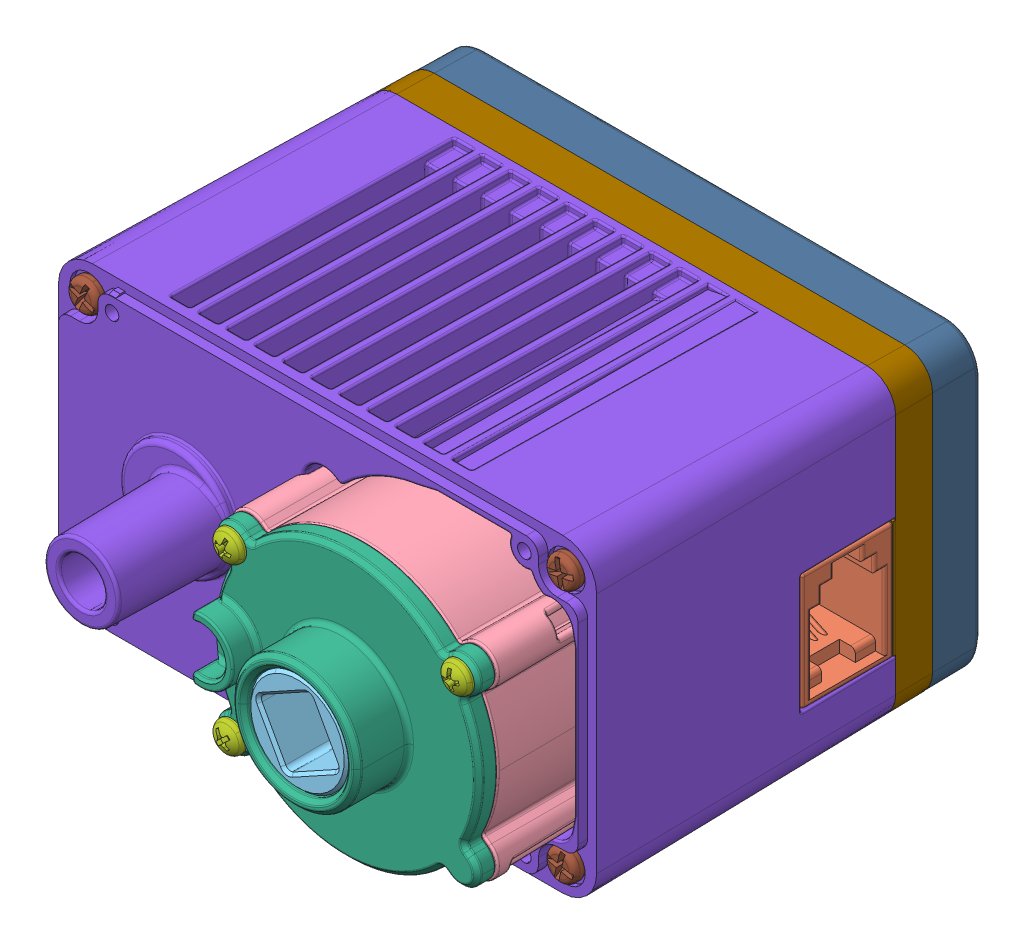
SolidWorks assembly V5 Smart Motor (276-4840), configuration Default. Lengths in mm.
Overall size (59.01 35.33 59.91).
20 component instances, 12 part files, 0 mates.
Components (placement in the parent):
- V5 Smart Motor (276-4840).step-1: V5 Smart Motor (276-4840).step [Default] at origin size (59.01 35.33 59.91)
  - 276-4840-900 Rev6_Instruction.step-1: 276-4840-900 Rev6_Instruction.step [Default] at (-14.3 0 -17.2) size (52.79 15.94 38.15)
    - 276-4840-901 Rev6.step-1: 276-4840-901 Rev6.step [Default] at (10.75 -10.05 17.8) x (-1 0 0) z (0 0 1) size (49.9 1.6 38.15)
    - 276-4840-902 Rev2.step-1: 276-4840-902 Rev2.step [Default] at (31.25 -9.25 6.2) x (0 0 -1) z (0 -1 0) size (10.35 11.39 15.94)
    - 276-4840-022 Rev4.step-1: 276-4840-022 Rev4.step [Default] at (31.25 -9.25 6.2) x (0 0 -1) z (1 0 0) size (10.26 9.1 5.51)
  - 276-4840-110 Rev10_Instruction.step-1: 276-4840-110 Rev10_Instruction.step [Default] at (12.7 0 14.7) size (35.33 35.33 31.1)
    - 276-4840-061 Rev7_Ring_Gear_Fixed01 .6 Rev3.step-1: 276-4840-061 Rev7_Ring_Gear_Fixed01 .6 Rev3.step [Default] at origin size (28.79 28.39 24.6)
    - 276-4840-018 Rev6.step-1: 276-4840-018 Rev6.step [Default] at (0 0 6.7) x (-0.483174 0.875524 0) z (0 0 1) size (26 26 12.3)
    - 276-4840-059 Rev2.step-1: 276-4840-059 Rev2.step [Default] at (0 0 10.3) size (28.4 28.4 8.5)
    - 276-4840-062 Rev1.step-1: 276-4840-062 Rev1.step [Default] at (-12.1353 8.8168 12.3) x (0.956835 -0.290632 0) z (-0.290632 -0.956835 0) size (3.2 6.56 3.2)
    - 276-4840-062 Rev1.step-2: 276-4840-062 Rev1.step [Default] at (12.1353 8.8168 12.3) x (0.978427 0.206591 0) z (0.206591 -0.978427 0) size (3.2 6.56 3.2)
    - 276-4840-062 Rev1.step-3: 276-4840-062 Rev1.step [Default] at (-12.1353 -8.8168 12.3) x (0.72563 0.688086 0) z (0.688086 -0.72563 0) size (3.2 6.56 3.2)
  - 276-4840-001 Rev38.step-1: 276-4840-001 Rev38.step [Default] at origin size (57.3 33 46.9)
  - 276-4840-005 Rev27.step-1: 276-4840-005 Rev27.step [Default] at (0 0 -17.95) size (56.17 31.87 12.9)
  - 276-4840-004 Rev16.step-1: 276-4840-004 Rev16.step [Default] at (0 0 -19.2) size (56.01 31.71 9.21)
  - 276-4840-009 Rev3.step-1: 276-4840-009 Rev3.step [Default] at (25.45 13.5 15.7) x (0.19987 -0.979823 0) z (-0.979823 -0.19987 0) size (3.4 41.31 4.34)
  - 276-4840-009 Rev3.step-2: 276-4840-009 Rev3.step [Default] at (-25.45 -13.5 15.7) x (-0.998855 0.047836 0) z (0.047836 0.998855 0) size (3.4 41.31 4.34)
  - 276-4840-009 Rev3.step-3: 276-4840-009 Rev3.step [Default] at (25.45 -13.5 15.7) x (-0.975374 0.220559 0) z (0.220559 0.975374 0) size (3.4 41.31 4.34)
  - 276-4840-009 Rev3.step-4: 276-4840-009 Rev3.step [Default] at (-25.45 13.5 15.7) x (-0.922256 0.38658 0) z (0.38658 0.922256 0) size (3.4 41.31 4.34)
  - 276-4840-025 Rev19.step-1: 276-4840-025 Rev19.step [Default] at (12.7 0 -22.63) x (-0.993315 0.115437 0) z (0 0 1) size (14.82 14.83 35.18)
